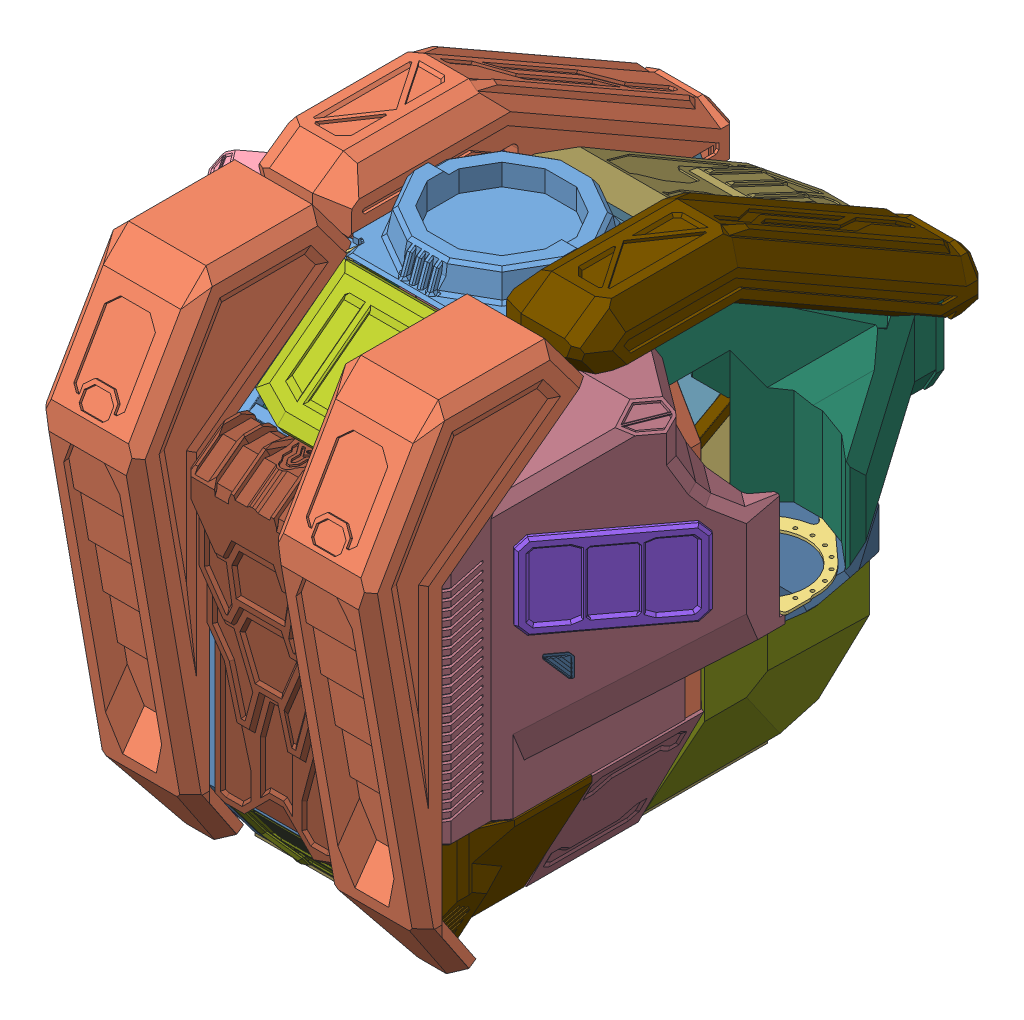
SolidWorks assembly Assemblage1_cockpit_v2, configuration Défaut. Lengths in mm.
Overall size (2088.81 2085.8 2703.64).
117 component instances, 75 part files, 251 mates.
Components (placement in the parent):
- cockpit_segmentLAT_0-1: cockpit_segmentLAT_0 [Défaut] at origin size (80 1780 1700)
- cockpit_segmentLAT_0-2: cockpit_segmentLAT_0 [Défaut] at (-580 0 0) size (80 1780 1700)
- cockpit_segmentFACE_0-1: cockpit_segmentFACE_0 [Défaut] at (-250 0 -10.6226) size (1180 1780 80)
- Manikin_sit-1: Manikin_sit [Default] at (-178.4008 -3076.5165 -521.6706) x (-0.998263 -0.006408 -0.058563) z (0.055728 0.219684 -0.973978) size (1056.52 1461.66 750.53)
  - Hips-1: Hips [Default] at (41.9716 15.4252 492.0452) x (0.998799 0.006411 -0.048571) z (0.047333 0.129538 0.990444) size (295.24 313.39 270.97)
  - Torso-1: Torso [Default] at (-29.1895 18.5281 -268.9557) x (0.995716 0.002037 -0.092438) z (0.092349 -0.071067 0.993187) size (460.89 555.97 263.41)
  - Head-2: Head [Default] at (-35.3994 3.8201 -64.7195) x (0.99996 -0.00842 0.002952) z (-0.003142 -0.022585 0.99974) size (157.49 285.21 225.45)
  - ArmLeftUpper-1: ArmLeftUpper [Default] at (-214.7655 17.6745 53.5906) x (0.983726 -0.048483 -0.173009) z (0.172972 -0.004986 0.984914) size (245.85 241.52 164.39)
  - LegLeftUpper-1: LegLeftUpper [Default] at (-298.9777 2948.9846 3668.472) x (0.995737 -0.057217 0.072354) z (0.044237 0.984495 0.169742) size (217.98 507.99 239.38)
  - ArmLeftFore-1: ArmLeftFore [Default] at (-737.1558 542.7506 1787.2483) x (0.68145 0.24029 0.691293) z (-0.69604 0.504688 0.510703) size (231.54 177.84 142.38)
  - ArmLeftHand-1: ArmLeftHand [Default] at (-1844.6946 922.3771 1244.5374) x (0.681315 -0.092916 0.72607) z (-0.527105 0.625983 0.574722) size (149.66 182.81 147.58)
  - LegLeftLower-1: LegLeftLower [Default] at (-393.4208 426.2264 1183.139) x (0.993791 -0.108531 0.024512) z (0.002157 0.239057 0.971003) size (171.81 443.68 193.78)
  - LegLeftFoot-1: LegLeftFoot [Default] at (-391.5322 345.3545 592.5292) x (0.993832 -0.110241 0.012061) z (-0.008622 0.031619 0.999463) size (154.71 147.12 252.53)
  - ArmRightUpper-1: ArmRightUpper [Default] at (-159.9752 -1.6557 34.3462) x (0.996289 -0.036751 -0.077828) z (0.077852 -0.000762 0.996965) size (246.03 241.06 163.63)
  - ArmRightFore-1: ArmRightFore [Default] at (825.1854 461.6545 1579.8734) x (0.462392 -0.291151 -0.837511) z (0.842326 0.439225 0.312359) size (231.51 177.54 142.76)
  - ArmRightHand-1: ArmRightHand [Default] at (3018.6854 2700.9935 1785.6002) x (0.598772 0.378902 -0.705624) z (0.060688 0.857021 0.511696) size (149.56 182.72 147.2)
  - LegRightUpper-1: LegRightUpper [Default] at (121.5915 3105.6896 3713.3645) x (0.987695 0.156074 -0.009999) z (-0.153555 0.97991 0.127269) size (216.84 507.94 244.77)
  - LegRightLower-1: LegRightLower [Default] at (672.1591 446.131 902.2036) x (0.976643 0.210274 0.044195) z (-0.073882 0.135492 0.98802) size (171.15 451.19 193.59)
  - LegRightFoot-1: LegRightFoot [Default] at (695.8533 419.9505 536.4877) x (0.976144 0.210831 0.051905) z (-0.054843 0.008108 0.998462) size (155.81 152.18 252.53)
- cockpit_segment_40x40_0-1: cockpit_segment_40x40_0 [Défaut] at (80 1283.2129 -10) size (258 40 730)
- cockpit_segment_40x40_0-2: cockpit_segment_40x40_0 [Défaut] at (-580 1323.2129 -10) x (-1 0 0) z (0 0 1) size (258 40 730)
- cockpit_segment_40x40_0-3: cockpit_segment_40x40_0 [Défaut] at (80 960 -10) size (258 40 730)
- cockpit_segment_40x40_0-4: cockpit_segment_40x40_0 [Défaut] at (-580 1000 -10) x (-1 0 0) z (0 0 1) size (258 40 730)
- cockpit_segmentFACE_0-2: cockpit_segmentFACE_0 [Défaut] at (-250 0 333.3333) size (1180 1780 80)
- cockpit_poutre40x80x500-5: cockpit_poutre40x80x500 [Défaut] at (-500 250 920) x (0 1 0) z (1 0 0) size (80 40 500)
- cockpit_poutre40x80x500-6: cockpit_poutre40x80x500 [Défaut] at (0 1330 920) x (0 -1 0) z (-1 0 0) size (80 40 500)
- cockpit_poutre40x80x500-7: cockpit_poutre40x80x500 [Défaut] at (-500 -40 -436.5685) x (0 0 -1) z (1 0 0) size (80 40 500)
- cockpit_poutre40x40x366-1: cockpit_poutre40x40x366 [Défaut] at (-840 1270.6802 69.3333) size (40 40 264)
- cockpit_poutre40x40x366-2: cockpit_poutre40x40x366 [Défaut] at (-840 440.3702 69.3333) size (40 40 264)
- cockpit_poutre40x40x366-3: cockpit_poutre40x40x366 [Défaut] at (300 1270.6802 69.3774) size (40 40 264)
- cockpit_poutre40x40x366-4: cockpit_poutre40x40x366 [Défaut] at (300 440.3702 69.3774) size (40 40 264)
- cockpit_poutre40x40x366-5: cockpit_poutre40x40x366 [Défaut] at (-840 960 67.3333) size (40 40 264)
- cockpit_poutre40x40x366-6: cockpit_poutre40x40x366 [Défaut] at (300 960 69.3774) size (40 40 264)
- bras_fixation_1-1: bras_fixation_1 [Défaut] at (340 990 512.9113) size (615.49 10 1037.05)
- bras_fixation_1-2: bras_fixation_1 [Défaut] at (-840 1000 512.9113) x (-1 0 0) z (0 0 1) size (615.49 10 1037.05)
- cockpit_poutre40x80x500-8: cockpit_poutre40x80x500 [Défaut] at (-500 396.2581 380) x (0 1 0) z (1 0 0) size (80 40 500)
- traverse_pente1-1: traverse_pente1 [Défaut] at (338 209.1038 -10.6226) x (-1 0 0) z (0 0 -1) size (257.78 292.58 728.37)
- traverse_pente1_sym-1: traverse_pente1_sym [Défaut] at (-838 209.1038 -10.6226) size (257.78 292.58 733.7)
- cockpit_poutre40x80x500-9: cockpit_poutre40x80x500 [Défaut] at (0 1340.3258 816.6212) x (0 0.90883 0.417168) z (-1 0 0) size (80 40 500)
- cockpit_segment_40x40_1_soutien_bras-1: cockpit_segment_40x40_1_soutien_bras [Défaut] at (-840 990 69.3774) x (0 -1 0) z (1 0 0) size (350 80 400)
- cockpit_segment_40x40_1_soutien_bras-2: cockpit_segment_40x40_1_soutien_bras [Défaut] at (340 990 -10.6226) x (0 -1 0) z (-1 0 0) size (350 80 400)
- cockpit_segment_40x40_2_back-1: cockpit_segment_40x40_2_back [Défaut] at (80 1310.6802 413.3333) x (1 0 0) z (0 0 -1) size (260 40 546)
- cockpit_segment_40x40_2_back-2: cockpit_segment_40x40_2_back [Défaut] at (-580 1270.6802 413.3333) x (-1 0 0) z (0 0 -1) size (260 40 546)
- attache_porte-1: attache_porte [Défaut] at (-500 1641.4369 -183.108) x (0 0.496139 0.868243) z (-1 0 0) size (198.66 73.18 10)
- attache_porte-2: attache_porte [Défaut] at (80 1641.4369 -183.108) x (0 0.496139 0.868243) z (-1 0 0) size (198.66 73.18 10)
- attache_porte-3: attache_porte [Défaut] at (-570 1641.4369 -183.108) x (0 0.496139 0.868243) z (-1 0 0) size (198.66 73.18 10)
- attache_porte-4: attache_porte [Défaut] at (10 1641.4369 -183.108) x (0 0.496139 0.868243) z (-1 0 0) size (198.66 73.18 10)
- axeO20.25_700-1: axeO20.25_700 [Défaut] at (-600 1702.1061 -146.8375) x (0 0.072457 -0.997372) z (1 0 0) size (20 20 700)
- Capot-1: Capot [Défaut] at (-480 1702.1061 -146.8375) x (-1 0 0) z (0 -0.505329 -0.862927) size (560 946.97 1454.08)
  - Capot1-1: Capot1 [Défaut] at origin size (10 749.16 1208.3)
  - Capot1-2: Capot1 [Défaut] at (-470 0 0) size (10 749.16 1208.3)
  - cockpit_poutre40x40x480-1: cockpit_poutre40x40x480 [Défaut] at (10 -20 40) x (0 0 1) z (-1 0 0) size (40 40 480)
  - cockpit_poutre40x40x480-2: cockpit_poutre40x40x480 [Défaut] at (10 -32.3205 751.7543) x (0 0.866025 0.5) z (-1 0 0) size (40 40 480)
  - cockpit_poutre40x40x480-3: cockpit_poutre40x40x480 [Défaut] at (10 -683.1793 1118.6603) x (0 -0.866025 0.5) z (-1 0 0) size (40 40 480)
  - Capot2-1: Capot2 [Défaut] at (-230 -26.9447 40) x (-1 0 0) z (0 0 -1) size (560 161.69 1100)
  - Capot3-1: Capot3 [Défaut] at (20 -892.9701 1297.518) x (-1 0 0) z (0 -0.5 -0.866025) size (500 906.77 276.51)
  - Capot4-1: Capot4 [Défaut] at (-470 0 0) x (0 0 -1) z (1 0 0) size (133 66 480)
- deco_torse1-1: deco_torse1 [Défaut] at (277.9178 1000 -180) size (738.18 710 1099)
- deco_torse2RIGHT-1: deco_torse2RIGHT [Défaut] at (336.2329 150 -15) size (343.72 998.15 825)
- deco_torse2LEFT-1: deco_torse2LEFT [Défaut] at (-173.0822 150 -15) size (343.72 998.15 825)
- deco_torse3_upRIGHT-1: deco_torse3_upRIGHT [Défaut] at (40.1918 1340 -57.5) x (0 0 -1) z (1 0 0) size (1491.8 695.65 350)
- deco_headcollar-1: deco_headcollar [Défaut] at (-540 1740 423.19) size (580 120 645)
- deco_torse4_back-1: deco_torse4_back [Défaut] at (0 250 960) size (370 1970 842.42)
  - deco_torse4_back-1: deco_torse4_back [Défaut] at origin size (370 1970 842.42)
- deco_torse4_back-2: deco_torse4_back [Défaut] at (-870 250 960) size (370 1970 842.42)
  - deco_torse4_back-1: deco_torse4_back [Défaut] at origin size (370 1970 842.42)
- attache_porte2-2: attache_porte2 [Défaut] at (0 1653 529.3333) x (0 0.6 -0.8) z (1 0 0) size (145 61.12 10)
- attache_porte2-4: attache_porte2 [Défaut] at (-510 1653 529.3333) x (0 0.6 -0.8) z (1 0 0) size (145 61.12 10)
- deco_torse5_back-1: deco_torse5_back [Défaut] at (-674.9206 1000 214) x (-1 0 0) z (0 0 -1) size (654 1290 891)
- deco_torse1_sym-1: deco_torse1_sym [Défaut] at (-238.4658 1000 -180) size (738.18 710 1099)
- axeO20_520-1: axeO20_520 [Défaut] at (10 1717.0991 489.9076) x (0 0 1) z (-1 0 0) size (20 20 520)
- écoutille1-1: écoutille1 [Défaut] at (-495 1713.4141 461.8644) x (0 -0.608956 0.793204) z (-1 0 0) size (485 60 490)
- back_trap-1: back_trap [Défaut] at (-1165.1221 1068.7153 290.3244) x (0.600343 0 0.799743) z (-0.799743 0 0.600343) size (530 320 30)
- deco_torse6_airvent-1: deco_torse6_airvent [Défaut] at (-834.9206 990 -10.6226) x (0 -1 0) z (1 0 0) size (382 611.74 504.34)
- airvent-1: airvent [Défaut] at (-958.7971 986.7153 581.836) x (0 -1 0) z (-0.600343 0 -0.799743) size (85 14 85)
- deco_torse7_dos-1: deco_torse7_dos [Défaut] at (0 230 960) x (-1 0 0) z (0 0 -1) size (500 1212.5 230)
- plancher-1: plancher [Défaut] at (-580 -50 740.5405) size (660 10 1260)
- deco_torse8_lateralinferieur-1: deco_torse8_lateralinferieur [Défaut] at (-599.1619 -30.8347 -6.6667) x (0 0 1) z (-0.890435 -0.455111 0) size (420 540 10)
- deco_torse8_lateralinferieur-2: deco_torse8_lateralinferieur [Défaut] at (99.1619 -30.8347 413.3333) x (0 0 -1) z (0.890435 -0.455111 0) size (420 540 10)
- attache_porte-5: attache_porte [Défaut] at (0 100.474 -657.0426) x (0 -0.707107 0.707107) z (1 0 0) size (198.66 73.18 10)
- attache_porte-6: attache_porte [Défaut] at (-510 100.474 -657.0426) x (0 -0.707107 0.707107) z (1 0 0) size (198.66 73.18 10)
- axeO20_520-2: axeO20_520 [Défaut] at (10 32.3991 -638.0132) x (0 0 1) z (-1 0 0) size (20 20 520)
- internalpanel1_back-1: internalpanel1_back [Défaut] at (-580 1402.9178 801.3393) x (1 0 0) z (0 0.417168 -0.90883) size (660 1010 10)
- internalpanel2_side-1: internalpanel2_side [Défaut] at (300 450 -10.6226) x (0 0 1) z (-1 0 0) size (424 850 10)
- internalpanel2_side-2: internalpanel2_side [Défaut] at (-800 450 413.3774) x (0 0 -1) z (1 0 0) size (424 850 10)
- internalpanel3_upside-1: internalpanel3_upside [Défaut] at (-799.2967 1301.2231 413.3774) x (0 0 -1) z (0.866906 -0.498471 0) size (424 460 10)
- internalpanel3_upside-2: internalpanel3_upside [Défaut] at (299.2967 1301.2231 -10.6226) x (0 0 1) z (-0.866906 -0.498471 0) size (424 460 10)
- internalpanel4_downside-1: internalpanel4_downside [Défaut] at (70 0 -10.6226) x (0 0 1) z (-0.890435 0.455111 0) size (424 503 10)
- internalpanel4_downside-2: internalpanel4_downside [Défaut] at (-570 0 413.3333) x (0 0 -1) z (0.890435 0.455111 0) size (424 503 10)
- internalpanel5_downback-1: internalpanel5_downback [Défaut] at (80 0 380) x (-1 0 0) z (0 0 -1) size (660 485 10)
- internalpanel6_floor-1: internalpanel6_floor [Défaut] at (80 0 -500) x (-1 0 0) z (0 1 0) size (660 870 10)
- sparco style race seat 1-1: sparco style race seat 1 [Default] at (-243.2192 277.46 345.725) x (0 0 1) z (-1 0 0) size (757.44 888.09 564.73)
- internalpanel7_frontLEFT-2: internalpanel7_frontLEFT [Défaut] at (13.6774 450 -703.8176) x (0.381763 0 0.92426) z (-0.92426 0 0.381763) size (750 1100 10)
- internalpanel8_frontRIGHT-1: internalpanel8_frontRIGHT [Défaut] at (-1086.3226 450 682.5725) x (0.381763 0 -0.92426) z (0.92426 0 0.381763) size (750 1100 10)
- internalpanel9_frontLup-1: internalpanel9_frontLup [Défaut] at (288.8206 1299.3811 -10.6226) x (-0.291598 -0.167669 -0.941731) z (0.816393 0.469426 -0.336366) size (736.22 460 3)
- internalpanel9_frontLup-2: internalpanel9_frontLup [Défaut] at (-791.2698 1300.7894 -11.6317) x (0.291598 -0.167669 -0.941731) z (0.816393 -0.469426 0.336366) size (736.22 460 3)
- internalpanel10_backsideLEFT-1: internalpanel10_backsideLEFT [Défaut] at (-580 485 380) x (0 0 -1) z (1 0 0) size (374.1 815 210)
- internalpanel10.5_backsideLEFT-1: internalpanel10.5_backsideLEFT [Défaut] at (-580 485 380) x (-1 0 0) z (0 0 -1) size (210 1220 10)
- internalpanel10_backsideRIGHT-1: internalpanel10_backsideRIGHT [Défaut] at (500 485 388.3406) x (0 0 -1) z (1 0 0) size (374.1 815 210)
- internalpanel10.5_backsideRIGHT-1: internalpanel10.5_backsideRIGHT [Défaut] at (80 485 388.3406) x (-1 0 0) z (0 0 -1) size (210 1220 10)
- deco_torse6_airventRIGHT-1: deco_torse6_airventRIGHT [Défaut] at (-281.076 990 -304.901) x (0 -1 0) z (0.628361 0 0.777922) size (382 438.89 781.29)
- internalpanel11_backsideUPLEFT-1: internalpanel11_backsideUPLEFT [Défaut] at (-800 1310.6802 413.3774) x (0 0 -1) z (1 0 0) size (385 365.22 210)
- internalpanel11_backsideUPRIGHT-1: internalpanel11_backsideUPRIGHT [Défaut] at (-140 1312.1 413.3333) x (0 0 -1) z (1 0 0) size (385 365.22 210)
- deco_torse5_backRIGHT-1: deco_torse5_backRIGHT [Défaut] at (1294 1000 214) x (-1 0 0) z (0 0 -1) size (654 1290 891)
- airvent-2: airvent [Défaut] at (457.8765 986.7153 581.836) x (-0.600343 0 0.799743) z (0 1 0) size (85 14 85)
- back_trap-2: back_trap [Défaut] at (358.0266 1068.7153 698.1932) x (0.600343 0 -0.799743) z (0.799743 0 0.600343) size (530 320 30)
- front_trapLEFT-1: front_trapLEFT [Défaut] at (-238.4658 1000 -910) x (-1 0 0) z (0 0 -1) size (311.73 350 50)
- front_trapRIGHT-1: front_trapRIGHT [Défaut] at (277.9178 1000 -910) x (-1 0 0) z (0 0 -1) size (311.73 350 50)
- deco_torse9_backbas-1: deco_torse9_backbas [Défaut] at (-500 -41.7099 725.6986) x (1 0 0) z (0 -0.603443 0.797406) size (500 371.41 25)
- deco_torse10_backbassideLEFT-1: deco_torse10_backbassideLEFT [Défaut] at (-855 -40 413.3333) size (275 490 530)
- deco_torse10_backbassideRIGHT-1: deco_torse10_backbassideRIGHT [Défaut] at (-195 -40 413.3333) size (275 490 530)
- écoutille2-1: écoutille2 [Défaut] at (0 -20.8559 -595.7178) x (-1 0 0) z (0 -0.36413 -0.931348) size (500 589.73 150)
- deco_torse3_upLEFT-1: deco_torse3_upLEFT [Défaut] at (-540.1918 1340 -57.5) x (0 0 -1) z (1 0 0) size (1491.8 695.65 350)
- attache_verin_cokpitepaul-1: attache_verin_cokpitepaul [Défaut] at (-739.6995 1260.6802 553.842) x (0.707107 0 -0.707107) z (0 1 0) size (92.03 103.34 10)
- attache_verin_cokpitepaul-2: attache_verin_cokpitepaul [Défaut] at (-739.6995 1190.6802 553.842) x (0.707107 0 -0.707107) z (0 1 0) size (92.03 103.34 10)
- attache_verin_cokpitepaul-3: attache_verin_cokpitepaul [Défaut] at (239.6995 1270.6802 553.842) x (-0.707107 0 -0.707107) z (0 -1 0) size (92.03 103.34 10)
- attache_verin_cokpitepaul-4: attache_verin_cokpitepaul [Défaut] at (119.4914 1190.6802 433.6338) x (0.707107 0 0.707107) z (0 1 0) size (92.03 103.34 10)
Mates (geometry in assembly coordinates):
- Distance1: distance = 500 mm anti-aligned: plane of cockpit_segmentLAT_0-1 through (0 0 0) normal (-1 0 0); plane of cockpit_segmentLAT_0-2 through (-500 0 0) normal (1 0 0)
- Coïncidente2: coincident aligned: plane of cockpit_segmentLAT_0-1 through (80 0 -740) normal (0 0 -1); plane of cockpit_segmentLAT_0-2 through (-500 0 -740) normal (0 0 -1)
- Coïncidente3: coincident aligned: plane of cockpit_segmentLAT_0-2 through (-500 1740 0) normal (0 1 0); plane of cockpit_segmentLAT_0-1 through (80 1740 0) normal (0 1 0)
- Coïncidente4: coincident aligned: plane of cockpit_segmentLAT_0-2 through (-500 1740 0) normal (0 1 0); plane of cockpit_segmentFACE_0-1 through (-593.1411 1740 69.3774) normal (0 1 0)
- Coïncidente5: coincident: line of cockpit_segmentLAT_0-1 through (78 1740 -10.6226) axis (-1 0 0); plane of cockpit_segmentFACE_0-1 through (-250 0 -10.6226) normal (0 0 -1)
- Distance2: distance = 250 mm: point of cockpit_segmentFACE_0-1; plane of cockpit_segmentLAT_0-2 through (-500 0 0) normal (1 0 0)
- Coïncidente7: coincident anti-aligned: plane of cockpit_segmentLAT_0-1 through (80 0 0) normal (1 0 0); plane of cockpit_segment_40x40_0-1 through (80 1323.2129 -619.9611) normal (-1 0 0)
- Coïncidente8: coincident: plane of cockpit_segmentLAT_0-1 through (80 0 -740) normal (0 0 -1); line of cockpit_segment_40x40_0-1 through (80 1321.2129 -740) axis (0 -1 0)
- Coïncidente9: coincident: line of cockpit_segmentLAT_0-1 through (78 1323.2129 -740) axis (-1 0 0); plane of cockpit_segment_40x40_0-1 through (80 1323.2129 -10) normal (0 1 0)
- Coïncidente11: coincident anti-aligned: plane of cockpit_segmentLAT_0-2 through (-580 0 0) normal (-1 0 0); plane of cockpit_segment_40x40_0-2 through (-580 1283.2129 -619.9611) normal (1 0 0)
- Coïncidente14: coincident: line of cockpit_segmentLAT_0-2 through (-502 1323.2129 -740) axis (-1 0 0); plane of cockpit_segment_40x40_0-2 through (-580 1323.2129 -10) normal (0 1 0)
- Coïncidente15: coincident: plane of cockpit_segmentLAT_0-2 through (-500 0 -740) normal (0 0 -1); line of cockpit_segment_40x40_0-2 through (-580 1285.2129 -740) axis (0 1 0)
- Coïncidente16: coincident anti-aligned: plane of cockpit_segmentLAT_0-1 through (80 0 0) normal (1 0 0); plane of cockpit_segment_40x40_0-3 through (80 1000 -619.9611) normal (-1 0 0)
- Coïncidente17: coincident: plane of cockpit_segmentLAT_0-1 through (80 0 -740) normal (0 0 -1); line of cockpit_segment_40x40_0-3 through (80 998 -740) axis (0 -1 0)
- Coïncidente18: coincident anti-aligned: plane of cockpit_segmentLAT_0-2 through (-580 0 0) normal (-1 0 0); plane of cockpit_segment_40x40_0-4 through (-580 960 -619.9611) normal (1 0 0)
- Coïncidente19: coincident: plane of cockpit_segmentLAT_0-2 through (-500 0 -740) normal (0 0 -1); line of cockpit_segment_40x40_0-4 through (-580 962 -740) axis (0 1 0)
- Coïncidente20: coincident aligned: plane of cockpit_segment_40x40_0-3 through (80 960 -10) normal (0 -1 0); plane of cockpit_segment_40x40_0-4 through (-580 960 -10) normal (0 -1 0)
- Coïncidente21: coincident aligned: plane of cockpit_segmentFACE_0-1 through (-593.1411 1740 69.3774) normal (0 1 0); plane of cockpit_segmentFACE_0-2 through (-593.1411 1740 413.3333) normal (0 1 0)
- Coïncidente22: coincident aligned: plane of cockpit_segmentFACE_0-1 through (-840 1310.6802 69.3774) normal (-1 0 0); plane of cockpit_segmentFACE_0-2 through (-840 1310.6802 413.3333) normal (-1 0 0)
- Coïncidente23: coincident: line of cockpit_segmentLAT_0-1 through (78 1740 413.3333) axis (-1 0 0); plane of cockpit_segmentFACE_0-2 through (-250 0 413.3333) normal (0 0 1)
- Coïncidente25: coincident aligned: plane of cockpit_segmentLAT_0-2 through (-500 -40 0) normal (0 -1 0); plane of cockpit_poutre40x80x500-7 through (0 -40 -438.5685) normal (0 -1 0)
- Coïncidente26: coincident anti-aligned: plane of cockpit_segmentLAT_0-2 through (-500 0 0) normal (1 0 0); plane of cockpit_poutre40x80x500-7 through (-500 -38 -438.5685) normal (-1 0 0)
- Coïncidente27: coincident: line of cockpit_segmentLAT_0-2 through (-502 -40 -516.5685) axis (-1 0 0); plane of cockpit_poutre40x80x500-7 through (0 -38 -516.5685) normal (0 0 -1)
- Coïncidente35: coincident aligned: plane of cockpit_segmentFACE_0-1 through (-840 1310.6802 69.3774) normal (-1 0 0); plane of cockpit_poutre40x40x366-1 through (-840 1272.6802 333.3333) normal (-1 0 0)
- Coïncidente36: coincident aligned: plane of cockpit_segmentFACE_0-1 through (-840 1310.6802 69.3774) normal (-1 0 0); plane of cockpit_poutre40x40x366-2 through (-840 442.3702 333.3333) normal (-1 0 0)
- Coïncidente37: coincident: line of cockpit_segmentFACE_0-1 through (-840 1310.6802 67.3774) axis (0 0 -1); plane of cockpit_poutre40x40x366-1 through (-838 1310.6802 333.3333) normal (0 1 0)
- Coïncidente38: coincident: line of cockpit_segmentFACE_0-1 through (-840 440.3702 67.3774) axis (0 0 -1); plane of cockpit_poutre40x40x366-2 through (-838 440.3702 333.3333) normal (0 -1 0)
- Coïncidente39: coincident anti-aligned: plane of cockpit_segmentFACE_0-2 through (-250 0 333.3333) normal (0 0 -1); plane of cockpit_poutre40x40x366-1 through (-838 1272.6802 333.3333) normal (0 0 1)
- Coïncidente40: coincident anti-aligned: plane of cockpit_segmentFACE_0-2 through (-250 0 333.3333) normal (0 0 -1); plane of cockpit_poutre40x40x366-2 through (-838 442.3702 333.3333) normal (0 0 1)
- Coïncidente41: coincident aligned: plane of cockpit_segmentFACE_0-2 through (340 1310.6802 413.3333) normal (1 0 0); plane of cockpit_poutre40x40x366-3 through (340 1272.6802 333.3774) normal (1 0 0)
- Coïncidente42: coincident: line of cockpit_segmentFACE_0-2 through (340 1310.6802 411.3333) axis (0 0 -1); plane of cockpit_poutre40x40x366-3 through (302 1310.6802 333.3774) normal (0 1 0)
- Coïncidente43: coincident anti-aligned: plane of cockpit_segmentFACE_0-1 through (-250 0 69.3774) normal (0 0 1); plane of cockpit_poutre40x40x366-3 through (302 1272.6802 69.3774) normal (0 0 -1)
- Coïncidente44: coincident aligned: plane of cockpit_segmentFACE_0-2 through (340 1310.6802 413.3333) normal (1 0 0); plane of cockpit_poutre40x40x366-4 through (340 442.3702 333.3774) normal (1 0 0)
- Coïncidente45: coincident: line of cockpit_segmentFACE_0-2 through (340 440.3702 411.3333) axis (0 0 -1); plane of cockpit_poutre40x40x366-4 through (302 440.3702 333.3774) normal (0 -1 0)
- Coïncidente47: coincident anti-aligned: plane of cockpit_segmentFACE_0-1 through (-250 0 69.3774) normal (0 0 1); plane of cockpit_poutre40x40x366-4 through (302 442.3702 69.3774) normal (0 0 -1)
- Distance3: distance = 1000 mm aligned: plane of cockpit_segment_40x40_0-3 through (80 960 -10) normal (0 -1 0); plane of cockpit_segmentLAT_0-1 through (80 -40 0) normal (0 -1 0)
- Coïncidente49: coincident aligned: plane of cockpit_segment_40x40_0-3 through (80 1000 -10) normal (0 1 0); plane of cockpit_poutre40x40x366-6 through (302 1000 333.3774) normal (0 1 0)
- Coïncidente50: coincident aligned: plane of cockpit_segment_40x40_0-4 through (-580 1000 -10) normal (0 1 0); plane of cockpit_poutre40x40x366-5 through (-838 1000 331.3333) normal (0 1 0)
- Coïncidente51: coincident aligned: plane of cockpit_segmentFACE_0-1 through (340 1310.6802 69.3774) normal (1 0 0); plane of cockpit_poutre40x40x366-6 through (340 962 333.3774) normal (1 0 0)
- Coïncidente52: coincident anti-aligned: plane of cockpit_segmentFACE_0-1 through (-250 0 69.3774) normal (0 0 1); plane of cockpit_poutre40x40x366-6 through (302 962 69.3774) normal (0 0 -1)
- Coïncidente53: coincident aligned: plane of cockpit_segmentFACE_0-1 through (-840 1310.6802 69.3774) normal (-1 0 0); plane of cockpit_poutre40x40x366-5 through (-840 962 331.3333) normal (-1 0 0)
- Coïncidente61: coincident aligned: plane of cockpit_segment_40x40_0-3 through (80 1000 -10) normal (0 1 0); plane of bras_fixation_1-1 through (540 1000 -47.0887) normal (0 1 0)
- Coïncidente63: coincident aligned: plane of cockpit_segment_40x40_0-4 through (-580 1000 -10) normal (0 1 0); plane of bras_fixation_1-2 through (-1040 1000 -47.0887) normal (0 1 0)
- Coïncidente70: coincident aligned: line of cockpit_segmentLAT_0-1 through (78 1330 960) axis (-1 0 0); plane of cockpit_poutre40x80x500-6 through (-500 1330 922) normal (0 1 0)
- Coïncidente71: coincident anti-aligned: plane of cockpit_segmentLAT_0-1 through (0 0 0) normal (-1 0 0); plane of cockpit_poutre40x80x500-6 through (0 1328 922) normal (1 0 0)
- Coïncidente72: coincident aligned: plane of cockpit_segmentLAT_0-1 through (80 0 960) normal (0 0 1); plane of cockpit_poutre40x80x500-6 through (-500 1328 960) normal (0 0 1)
- Coïncidente73: coincident aligned: plane of cockpit_segmentLAT_0-2 through (-500 0 960) normal (0 0 1); plane of cockpit_poutre40x80x500-5 through (0 252 960) normal (0 0 1)
- Coïncidente74: coincident anti-aligned: plane of cockpit_segmentLAT_0-2 through (-500 0 0) normal (1 0 0); plane of cockpit_poutre40x80x500-5 through (-500 252 922) normal (-1 0 0)
- Coïncidente75: coincident: line of cockpit_segmentLAT_0-1 through (78 250 960) axis (-1 0 0); plane of cockpit_poutre40x80x500-5 through (0 250 922) normal (0 -1 0)
- Coïncidente76: coincident aligned: plane of cockpit_segmentLAT_0-1 through (80 0 420) normal (0 0 1); plane of cockpit_poutre40x80x500-8 through (0 398.2581 420) normal (0 0 1)
- Coïncidente77: coincident anti-aligned: plane of cockpit_segmentLAT_0-2 through (-500 0 0) normal (1 0 0); plane of cockpit_poutre40x80x500-8 through (-500 398.2581 382) normal (-1 0 0)
- Coïncidente78: coincident: line of cockpit_segmentLAT_0-2 through (-502 476.2581 420) axis (-1 0 0); plane of cockpit_poutre40x80x500-8 through (0 476.2581 382) normal (0 1 0)
- Coïncidente83: coincident anti-aligned: plane of cockpit_segmentLAT_0-1 through (80 0 0) normal (1 0 0); plane of traverse_pente1-1 through (80 469.3117 -739.6226) normal (-1 0 0)
- Coïncidente86: coincident anti-aligned: plane of cockpit_segmentFACE_0-1 through (-250 0 -10.6226) normal (0 0 -1); plane of traverse_pente1-1 through (338 209.1038 -10.6226) normal (0 0 1)
- Coïncidente92: coincident: line of cockpit_segmentLAT_0-1 through (80 -38 -515.7401) axis (0 0.707107 -0.707107); point of traverse_pente1-1
- Coïncidente93: coincident anti-aligned: plane of cockpit_segmentFACE_0-1 through (-250 0 -10.6226) normal (0 0 -1); plane of traverse_pente1_sym-1 through (-835.8915 172.5363 -10.6226) normal (0 0 1)
- Coïncidente96: coincident anti-aligned: plane of cockpit_segmentLAT_0-2 through (-580 0 0) normal (-1 0 0); plane of traverse_pente1_sym-1 through (-580 469.3117 -739.6226) normal (1 0 0)
- Coïncidente98: coincident: line of cockpit_segmentLAT_0-2 through (-580 184.2599 -738) axis (0 -0.707107 0.707107); point of traverse_pente1_sym-1
- Coïncidente102: coincident aligned: plane of cockpit_segmentLAT_0-2 through (-500 -76.3537 166.3421) normal (0 -0.417168 0.90883); plane of cockpit_poutre40x80x500-9 through (-500 1342.1434 817.4555) normal (0 -0.417168 0.90883)
- Coïncidente103: coincident anti-aligned: plane of cockpit_segmentLAT_0-2 through (-500 0 0) normal (1 0 0); plane of cockpit_poutre40x80x500-9 through (-500 1342.9778 815.6379) normal (-1 0 0)
- Coïncidente108: coincident anti-aligned: plane of cockpit_segmentFACE_0-1 through (340 1310.6802 69.3774) normal (1 0 0); plane of cockpit_segment_40x40_1_soutien_bras-2 through (340 693.1507 69.3774) normal (-1 0 0)
- Coïncidente109: coincident anti-aligned: plane of bras_fixation_1-1 through (540 990 -47.0887) normal (0 -1 0); plane of cockpit_segment_40x40_1_soutien_bras-2 through (679.2563 990 69.3774) normal (0 1 0)
- Coïncidente110: coincident aligned: plane of cockpit_segmentFACE_0-1 through (-250 0 -10.6226) normal (0 0 -1); plane of cockpit_segment_40x40_1_soutien_bras-2 through (340 990 -10.6226) normal (0 0 -1)
- Coïncidente114: coincident anti-aligned: plane of cockpit_segmentFACE_0-2 through (-840 1310.6802 413.3333) normal (-1 0 0); plane of cockpit_segment_40x40_1_soutien_bras-1 through (-840 693.1507 -10.6226) normal (1 0 0)
- Coïncidente115: coincident anti-aligned: plane of bras_fixation_1-2 through (-1040 990 -47.0887) normal (0 -1 0); plane of cockpit_segment_40x40_1_soutien_bras-1 through (-1179.2563 990 -10.6226) normal (0 1 0)
- Coïncidente116: coincident aligned: plane of cockpit_segmentFACE_0-1 through (-250 0 -10.6226) normal (0 0 -1); plane of cockpit_segment_40x40_1_soutien_bras-1 through (-840 990 -10.6226) normal (0 0 -1)
- Coïncidente117: coincident anti-aligned: plane of cockpit_segmentFACE_0-2 through (-250 0 413.3333) normal (0 0 1); plane of cockpit_segment_40x40_2_back-2 through (-795.6964 1310.6802 413.3333) normal (0 0 -1)
- Coïncidente118: coincident anti-aligned: plane of cockpit_segmentLAT_0-2 through (-580 0 0) normal (-1 0 0); plane of cockpit_segment_40x40_2_back-2 through (-580 1310.6802 866.2957) normal (1 0 0)
- Coïncidente119: coincident aligned: plane of cockpit_poutre40x40x366-1 through (-838 1310.6802 333.3333) normal (0 1 0); plane of cockpit_segment_40x40_2_back-2 through (-580 1310.6802 413.3333) normal (0 1 0)
- Coïncidente121: coincident anti-aligned: plane of cockpit_segmentFACE_0-2 through (-250 0 413.3333) normal (0 0 1); plane of cockpit_segment_40x40_2_back-1 through (295.6964 1270.6802 413.3333) normal (0 0 -1)
- Coïncidente122: coincident anti-aligned: plane of cockpit_segmentLAT_0-1 through (80 0 0) normal (1 0 0); plane of cockpit_segment_40x40_2_back-1 through (80 1270.6802 866.2957) normal (-1 0 0)
- Coïncidente123: coincident aligned: plane of cockpit_poutre40x40x366-3 through (302 1310.6802 333.3774) normal (0 1 0); plane of cockpit_segment_40x40_2_back-1 through (80 1310.6802 413.3333) normal (0 1 0)
- Coïncidente124: coincident anti-aligned: plane of cockpit_poutre40x40x366-5 through (-840 962 331.3333) normal (-1 0 0); plane of bras_fixation_1-2 through (-840 990 512.9113) normal (1 0 0)
- Coïncidente125: coincident anti-aligned: plane of cockpit_poutre40x40x366-6 through (340 962 333.3774) normal (1 0 0); plane of bras_fixation_1-1 through (340 1000 512.9113) normal (-1 0 0)
- Coïncidente128: coincident: plane of cockpit_segmentFACE_0-2 through (-250 0 413.3333) normal (0 0 1); line of bras_fixation_1-2 through (-840 1000 413.3333) axis (0 -1 0)
- Coïncidente131: coincident: plane of cockpit_segmentFACE_0-2 through (-250 0 413.3333) normal (0 0 1); line of bras_fixation_1-1 through (340 990 413.3333) axis (0 1 0)
- Coaxiale1: concentric aligned: cylinder of attache_porte-3 through (-580 1702.1061 -146.8375) axis (1 0 0) radius 23.5; cylinder of attache_porte-4 through (0 1702.1061 -146.8375) axis (1 0 0) radius 23.5
- Coaxiale3: concentric aligned: cylinder of attache_porte-2 through (70 1702.1061 -146.8375) axis (1 0 0) radius 23.5; cylinder of attache_porte-3 through (-580 1702.1061 -146.8375) axis (1 0 0) radius 23.5
- Coaxiale4: concentric aligned: cylinder of attache_porte-1 through (-510 1702.1061 -146.8375) axis (1 0 0) radius 23.5; cylinder of attache_porte-3 through (-580 1702.1061 -146.8375) axis (1 0 0) radius 23.5
- Coïncidente132: coincident aligned: plane of cockpit_segmentLAT_0-2 through (-580 0 0) normal (-1 0 0); plane of attache_porte-3 through (-580 1702.1061 -146.8375) normal (-1 0 0)
- Coïncidente133: coincident aligned: plane of cockpit_segmentLAT_0-2 through (-500 0 0) normal (1 0 0); plane of attache_porte-1 through (-500 1702.1061 -146.8375) normal (1 0 0)
- Coïncidente134: coincident aligned: plane of cockpit_segmentLAT_0-1 through (80 0 0) normal (1 0 0); plane of attache_porte-2 through (80 1702.1061 -146.8375) normal (1 0 0)
- Coïncidente135: coincident aligned: plane of cockpit_segmentLAT_0-1 through (0 0 0) normal (-1 0 0); plane of attache_porte-4 through (0 1702.1061 -146.8375) normal (-1 0 0)
- Coïncidente140: coincident anti-aligned: plane of cockpit_segmentLAT_0-2 through (-500 1316.2682 -752.1532) normal (0 0.868243 -0.496139); plane of attache_porte-3 through (-580 1735.7033 -18.1418) normal (0 -0.868243 0.496139)
- Coaxiale5: concentric anti-aligned: cylinder of attache_porte-3 through (-580 1702.1061 -146.8375) axis (1 0 0) radius 23.5; cylinder of axeO20.25_700-1 through (100 1702.1061 -146.8375) axis (-1 0 0) radius 10
- Distance4: distance = 20 mm aligned: plane of attache_porte-3 through (-580 1702.1061 -146.8375) normal (-1 0 0); plane of axeO20.25_700-1 through (-600 1702.1061 -146.8375) normal (-1 0 0)
- Coïncidente145: coincident anti-aligned: line of cockpit_segmentLAT_0-1 through (78 1740 -10.6226) axis (-1 0 0); line of attache_porte-2 through (70 1740 -10.6226) axis (1 0 0)
